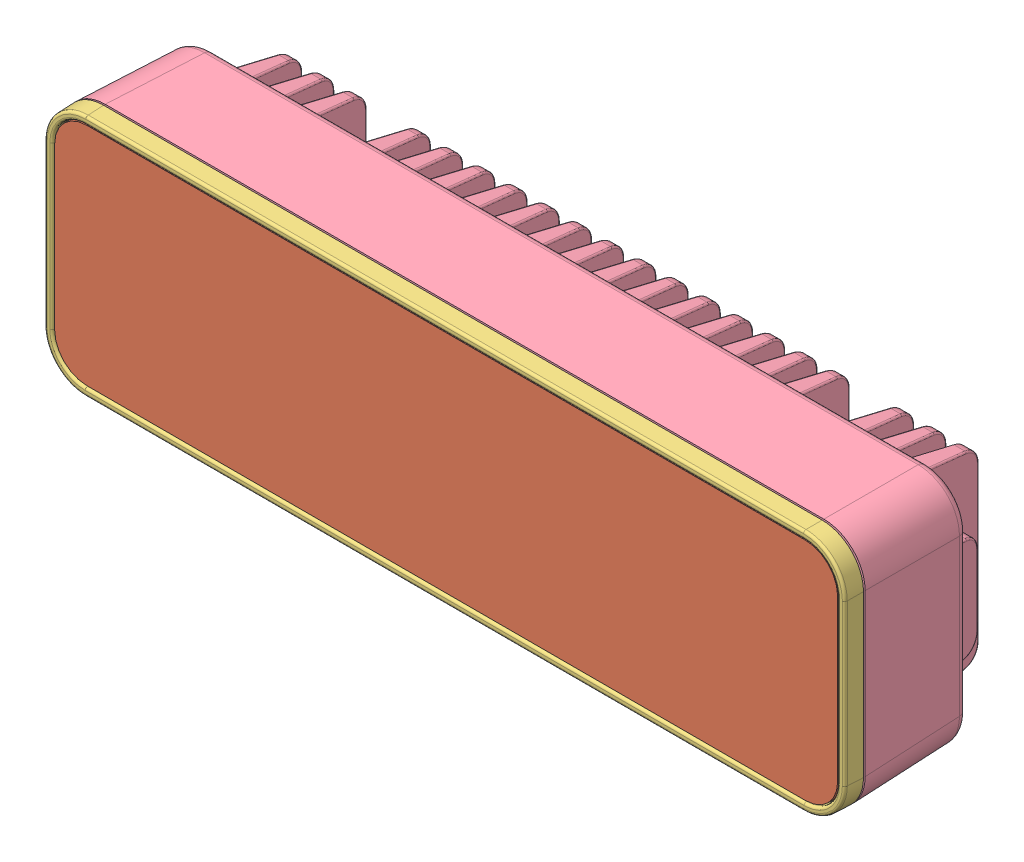
SolidWorks assembly OAK-D-Pro, configuration Default. Lengths in mm.
Overall size (97.03 29.53 23.13).
16 component instances, 10 part files, 0 mates.
Components (placement in the parent):
- OAK-D-Pro_enclosure.stp-1: OAK-D-Pro_enclosure.stp [Default] at origin size (97.03 29.53 23.13)
  - 609-00007_ASM.stp-1: 609-00007_ASM.stp [Default] at (44.5 -6.9862 9.1009) size (94.8 27.3 0.83)
    - D-PRO-LENS-ADHESIVE.stp-1: D-PRO-LENS-ADHESIVE.stp [Default] at origin size (94.2 26.7 0.2)
    - D-PRO-GLASS-LENS.stp-1: D-PRO-GLASS-LENS.stp [Default] at (0 0 0.23) size (94.8 27.3 0.6)
  - 606-00013-02.stp-1: 606-00013-02.stp [Default] at origin size (97.03 29.53 11.71)
  - 606-00014-02.stp-1: 606-00014-02.stp [Default] at origin size (97.03 29.53 20.74)
  - 611-00019.stp-1: 611-00019.stp [Default] at (82 -6.9862 7.6009) x (-1 0 0) z (0 0 -1) size (12 12 4)
  - 611-00019.stp-2: 611-00019.stp [Default] at (6.9999 -6.9862 7.6009) x (-1 0 0) z (0 0 -1) size (12 12 4)
  - 611-00018.stp-1: 611-00018.stp [Default] at (44.5 -6.9863 7.6009) x (-1 0 0) z (0 0 -1) size (12 12 2.5)
  - 611-00016.stp-1: 611-00016.stp [Default] at (63.25 -7.05 1.5009) size (17 10.2 1.6)
  - 612-00003.stp-1: 612-00003.stp [Default] at (58.5 -8 -1.3) size (22 15 1.5)
  - 612-00002.stp-1: 612-00002.stp [Default] at (30.43 -12.99 -1.3) size (10 10 0.5)
  - 602-00007.stp-1: 602-00007.stp [Default] at (73.8 -3.5 4.5) size (4.5 4.5 10.5)
  - 602-00007.stp-2: 602-00007.stp [Default] at (69.51 -21.99 4.5) size (4.5 4.5 10.5)
  - 602-00007.stp-3: 602-00007.stp [Default] at (15.75 -3.5 4.5) size (4.5 4.5 10.5)
  - 602-00007.stp-4: 602-00007.stp [Default] at (18.35 -21.99 4.5) size (4.5 4.5 10.5)
